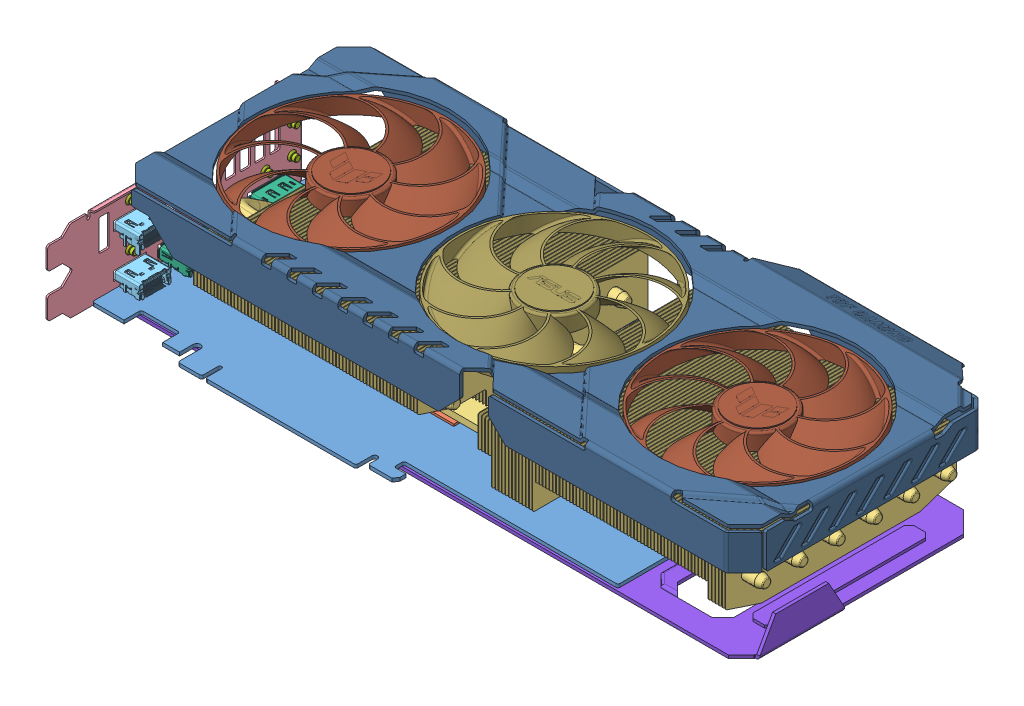
SolidWorks assembly ASUS TUF RX 6800, configuration Default. Lengths in mm.
Overall size (312.86 54.46 157.26).
24 component instances, 12 part files, 0 mates.
Components (placement in the parent):
- ASUS TUF RTX 3070 ti.stp-1: ASUS TUF RTX 3070 ti.stp [Default] at origin size (312.86 54.46 157.26)
  - PCB MSI.stp-1: PCB MSI.stp [Default] at origin size (240 1.6 129.85)
  - DIE and Chips.stp-1: DIE and Chips.stp [Default] at (-7 1.6 -3.6) size (97.5 4 74.8)
  - ASUS Cooler.stp-1: ASUS Cooler.stp [Default] at (-7 3.6 -3.6) x (-1 0 0) z (0 0 -1) size (281.94 30.71 109.44)
  - IO MSI.stp-1: IO MSI.stp [Default] at (-122 -1.2 86.6) x (0 0 -1) z (1 0 0) size (120.7 43.1 14.31)
  - HDMI Connector.stp-1: HDMI Connector.stp [Default] at (50.3 0.095 146.15) x (0 0 -1) z (0 1 0) size (15 12.15 8.38)
  - HDMI Connector.stp-2: HDMI Connector.stp [Default] at (50.3 20.495 146.15) x (0 0 -1) z (0 1 0) size (15 12.15 8.38)
  - displayport.stp-1: displayport.stp [Default] at (-120.2 4.98 26) x (0 0 1) z (-1 0 0) size (17.79 8.75 14.89)
  - displayport.stp-2: displayport.stp [Default] at (-120.2 4.98 4.5) x (0 0 1) z (-1 0 0) size (17.79 8.75 14.89)
  - displayport.stp-3: displayport.stp [Default] at (-120.2 4.98 -17) x (0 0 1) z (-1 0 0) size (17.79 8.75 14.89)
  - ISO 7046-1 - M3 x 4 - 4.8 - H.stp-1: ISO 7046-1 - M3 x 4 - 4.8 - H.stp [Default] at (-122 26.75 -28.9) x (1 0 0) z (0 -0.01976 0.999805) size (3.5 5 5)
  - ISO 7046-1 - M3 x 4 - 4.8 - H.stp-2: ISO 7046-1 - M3 x 4 - 4.8 - H.stp [Default] at (-122 13 -28.9) x (1 0 0) z (0 0.999805 0.01976) size (3.5 5 5)
  - ISO 7046-1 - M3 x 4 - 4.8 - H.stp-3: ISO 7046-1 - M3 x 4 - 4.8 - H.stp [Default] at (-122 13 4.85) x (1 0 0) z (0 0.999805 0.01976) size (3.5 5 5)
  - ISO 7046-1 - M3 x 4 - 4.8 - H.stp-4: ISO 7046-1 - M3 x 4 - 4.8 - H.stp [Default] at (-122 13 47.65) x (1 0 0) z (0 0.999805 0.01976) size (3.5 5 5)
  - ISO 7046-1 - M3 x 4 - 4.8 - H.stp-5: ISO 7046-1 - M3 x 4 - 4.8 - H.stp [Default] at (-122 33.4 47.65) x (1 0 0) z (0 0.999805 0.01976) size (3.5 5 5)
  - ISO 7046-1 - M3 x 4 - 4.8 - H.stp-6: ISO 7046-1 - M3 x 4 - 4.8 - H.stp [Default] at (-122 13 26) x (1 0 0) z (0 0.999805 0.01976) size (3.5 5 5)
  - ISO 7046-1 - M3 x 4 - 4.8 - H.stp-7: ISO 7046-1 - M3 x 4 - 4.8 - H.stp [Default] at (-122 13 -16.3) x (1 0 0) z (0 0.999805 0.01976) size (3.5 5 5)
  - ASUS Backplate.stp-1: ASUS Backplate.stp [Default] at (30.2 -2.5 -0.6) x (1 0 0) z (0 0 -1) size (298 15.51 115)
  - Conector 8 Pines a PCB en Codo.stp-1: Conector 8 Pines a PCB en Codo.stp [Default] at (90.15 11.6 -58.6) x (1 0 0) z (0 0 -1) size (18.4 12.4 19.94)
  - Conector 8 Pines a PCB en Codo.stp-2: Conector 8 Pines a PCB en Codo.stp [Default] at (109.55 11.6 -58.6) x (1 0 0) z (0 0 -1) size (18.4 12.4 19.94)
  - ASUS TUF Backplate - Kopie.stp-1: ASUS TUF Backplate - Kopie.stp [Default] at (29.2 47.6 -1.1) x (0 0 1) z (-1 0 0) size (127.06 30.93 298.38)
  - ASUS Fan 90mm.stp-1: ASUS Fan 90mm.stp [Default] at (-66 39.8 -1.6) x (0 0 1) z (-1 0 0) size (90 9.7 90)
  - ASUS Fan 90mm.stp-2: ASUS Fan 90mm.stp [Default] at (126 39.8 -1.6) x (0 0 1) z (-1 0 0) size (90 9.7 90)
  - ASUS Fan 90mm_1.stp-1: ASUS Fan 90mm_1.stp [Default] at (30 39.8 -1.6) size (90 9.66 90)
